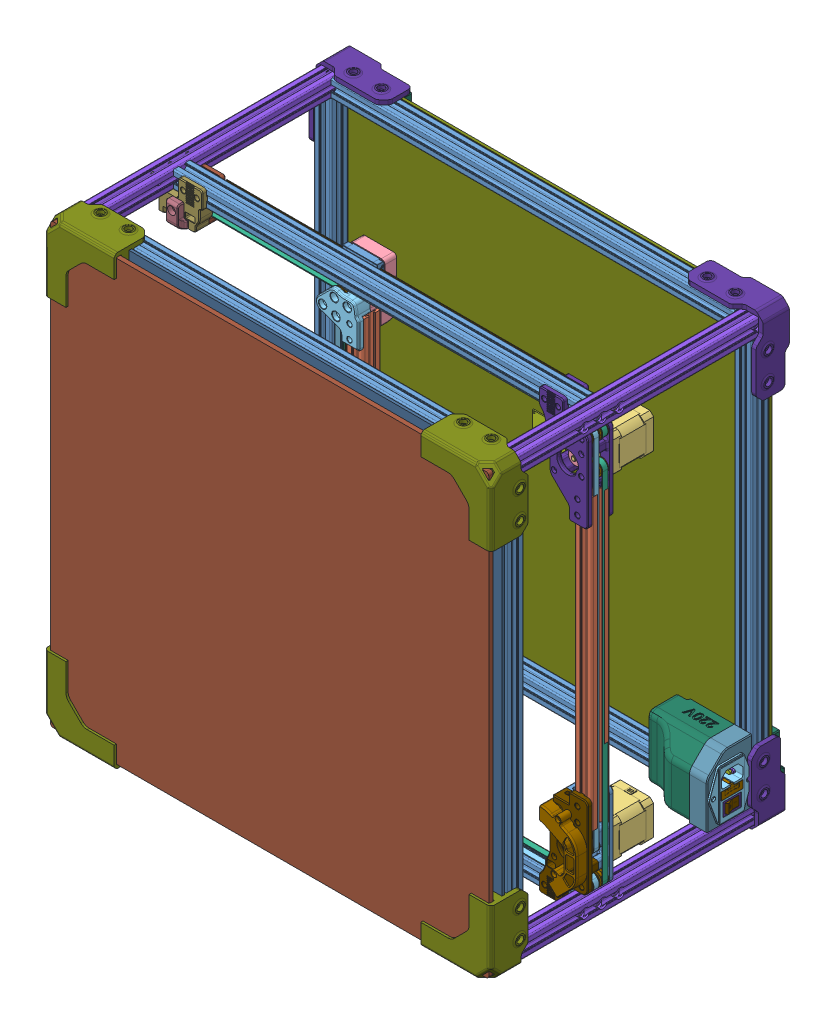
SolidWorks assembly Assem, configuration Default. Lengths in mm. (continued)
Mates (geometry in assembly coordinates): (continued)
- Concentric59: concentric anti-aligned: cylinder of F695 ZZ (1)^Idler Assembly (1)_1_XY Joint - Right_X Axis_Gantry_VORON2 v2.4 Assembly - Final(2)_VORON2 v2.4 Assembly - Final-19 through (240.5064 -184.1733 3) axis (0 0 1) radius 6.5; cylinder of F695 ZZ (1)^Idler Assembly (1)_1_XY Joint - Right_X Axis_Gantry_VORON2 v2.4 Assembly - Final(2)_VORON2 v2.4 Assembly - Final-20 through (240.5064 -184.1733 7) axis (0 0 -1) radius 6.5
- Concentric60: concentric aligned: cylinder of A Drive Frame-23^A Drive Frame_A Drive_Gantry_VORON2 v2.4 Assembly - Final(2)_VORON2 v2.4 Assembly - Final-1 through (240.5064 -184.1733 15) axis (0 0 -1) radius 2.7; cylinder of F695 ZZ (1)^Idler Assembly (1)_1_XY Joint - Right_X Axis_Gantry_VORON2 v2.4 Assembly - Final(2)_VORON2 v2.4 Assembly - Final-20 through (240.5064 -184.1733 7) axis (0 0 -1) radius 6.5
- Coincident93: coincident anti-aligned: plane of A Drive Frame-23^A Drive Frame_A Drive_Gantry_VORON2 v2.4 Assembly - Final(2)_VORON2 v2.4 Assembly - Final-1 through (220.1397 -181.8752 10) normal (0 0 -1); plane of M5 1mm Spacer (1)^Idler Assembly (1)_1_XY Joint - Right_X Axis_Gantry_VORON2 v2.4 Assembly - Final(2)_VORON2 v2.4 Assembly - Final-19 through (240.5064 -184.1733 10) normal (0 0 1)
- Coincident94: coincident anti-aligned: plane of B Drive Frame (1)^B Drive_Gantry_VORON2 v2.4 Assembly - Final(2)_VORON2 v2.4 Assembly - Final-1 through (225.0294 190.9774 -15) normal (0 0 -1); plane of NEMA17 Black^B Drive_Gantry_VORON2 v2.4 Assembly - Final(2)_VORON2 v2.4 Assembly - Final-1 through (204.0284 169.9764 -15) normal (0 0 1)
- Concentric61: concentric anti-aligned: cylinder of B Drive Frame (1)^B Drive_Gantry_VORON2 v2.4 Assembly - Final(2)_VORON2 v2.4 Assembly - Final-1 through (225.0294 190.9774 -16.6) axis (0 0 -1) radius 11.5; cylinder of NEMA17 Black^B Drive_Gantry_VORON2 v2.4 Assembly - Final(2)_VORON2 v2.4 Assembly - Final-1 through (225.0294 190.9774 -15.6) axis (0 0 1) radius 11
- Parallel3: parallel aligned: plane of B Drive Frame (1)^B Drive_Gantry_VORON2 v2.4 Assembly - Final(2)_VORON2 v2.4 Assembly - Final-1 through (248.0294 221.1733 -16.6) normal (1 0 0); plane of NEMA17 Black^B Drive_Gantry_VORON2 v2.4 Assembly - Final(2)_VORON2 v2.4 Assembly - Final-1 through (246.0294 174.1654 -25.161) normal (1 0 0)
- Concentric62: concentric anti-aligned: cylinder of B Drive Frame (1)^B Drive_Gantry_VORON2 v2.4 Assembly - Final(2)_VORON2 v2.4 Assembly - Final-1 through (240.5294 221.1733 15) axis (0 0 1) radius 2.7; cylinder of F695 ZZ (1)^Idler Assembly (1)_1_XY Joint - Right_X Axis_Gantry_VORON2 v2.4 Assembly - Final(2)_VORON2 v2.4 Assembly - Final-16 through (240.5294 221.1733 7) axis (0 0 -1) radius 6.5
- Coincident97: coincident anti-aligned: plane of A Drive Frame-24^A Drive Frame_A Drive_Gantry_VORON2 v2.4 Assembly - Final(2)_VORON2 v2.4 Assembly - Final-1 through (220.0147 -192 -15) normal (0 0 -1); plane of NEMA17 Black^B Drive_Gantry_VORON2 v2.4 Assembly - Final(2)_VORON2 v2.4 Assembly - Final-2 through (246.0304 -169.9764 -15) normal (0 0 1)
- Concentric63: concentric aligned: cylinder of A Drive Frame-24^A Drive Frame_A Drive_Gantry_VORON2 v2.4 Assembly - Final(2)_VORON2 v2.4 Assembly - Final-1 through (225.0294 -190.9774 -16.6) axis (0 0 1) radius 11.5; cylinder of NEMA17 Black^B Drive_Gantry_VORON2 v2.4 Assembly - Final(2)_VORON2 v2.4 Assembly - Final-2 through (225.0294 -190.9774 -15.6) axis (0 0 1) radius 11
- Parallel4: parallel aligned: plane of A Drive Frame-24^A Drive Frame_A Drive_Gantry_VORON2 v2.4 Assembly - Final(2)_VORON2 v2.4 Assembly - Final-1 through (248.0294 -221.1733 -16.6) normal (1 0 0); plane of NEMA17 Black^B Drive_Gantry_VORON2 v2.4 Assembly - Final(2)_VORON2 v2.4 Assembly - Final-2 through (246.0294 -174.1654 -25.161) normal (1 0 0)
- Concentric64: concentric anti-aligned: cylinder of NEMA17 Black^B Drive_Gantry_VORON2 v2.4 Assembly - Final(2)_VORON2 v2.4 Assembly - Final-2 through (225.0294 -190.9774 8.3401) axis (0 0 -1) radius 2.4956; cylinder of GT2 20T 6mm^B Drive_Gantry_VORON2 v2.4 Assembly - Final(2)_VORON2 v2.4 Assembly - Final-1 through (225.0294 -190.9774 -6.35) axis (0 0 1) radius 2.5
- Distance14: distance = 0.5 mm aligned: plane of GT2 20T 6mm^B Drive_Gantry_VORON2 v2.4 Assembly - Final(2)_VORON2 v2.4 Assembly - Final-1 through (225.0294 -190.9774 8.5) normal (0 0 -1); plane of F695 ZZ (1)^Idler Assembly (1)_1_XY Joint - Right_X Axis_Gantry_VORON2 v2.4 Assembly - Final(2)_VORON2 v2.4 Assembly - Final-20 through (240.5064 -184.1733 8) normal (0 0 -1)
- Concentric66: concentric aligned: cylinder of NEMA17 Black^B Drive_Gantry_VORON2 v2.4 Assembly - Final(2)_VORON2 v2.4 Assembly - Final-1 through (225.0294 190.9774 8.3401) axis (0 0 -1) radius 2.4956; cylinder of GT2 20T 6mm^B Drive_Gantry_VORON2 v2.4 Assembly - Final(2)_VORON2 v2.4 Assembly - Final-2 through (225.0294 190.9774 6.35) axis (0 0 -1) radius 2.5
- Distance15: distance = 0.5 mm aligned: plane of GT2 20T 6mm^B Drive_Gantry_VORON2 v2.4 Assembly - Final(2)_VORON2 v2.4 Assembly - Final-2 through (225.0294 190.9774 -1.5) normal (0 0 -1); plane of F695 ZZ (1)^Idler Assembly (1)_1_XY Joint - Right_X Axis_Gantry_VORON2 v2.4 Assembly - Final(2)_VORON2 v2.4 Assembly - Final-17 through (240.5064 184.1733 -2) normal (0 0 -1)
- Coincident102: coincident anti-aligned: plane of Front Idler B Bottom^Front Idler B_Gantry_VORON2 v2.4 Assembly - Final(2)_VORON2 v2.4 Assembly - Final-1 through (-220 227.6989 -10) normal (0 0 1); plane of M5 1mm Spacer (1)^Idler Assembly (1)_1_XY Joint - Right_X Axis_Gantry_VORON2 v2.4 Assembly - Final(2)_VORON2 v2.4 Assembly - Final-5 through (-219.5002 221.0003 -10) normal (0 0 -1)
- BeltMate1: belt = 13 : 12.22 mm: cylinder of GT2 20T 6mm^B Drive_Gantry_VORON2 v2.4 Assembly - Final(2)_VORON2 v2.4 Assembly - Final-2 through (225.0294 190.9774 6.35) axis (0 0 1) radius 6.11; cylinder of F695 ZZ (1)^Idler Assembly (1)_1_XY Joint - Right_X Axis_Gantry_VORON2 v2.4 Assembly - Final(2)_VORON2 v2.4 Assembly - Final-18 through (240.5064 184.1733 -7) axis (0 0 1) radius 6.5
- BeltMate2: belt = 13 : 13 mm: cylinder of F695 ZZ (1)^Idler Assembly (1)_1_XY Joint - Right_X Axis_Gantry_VORON2 v2.4 Assembly - Final(2)_VORON2 v2.4 Assembly - Final-18 through (240.5064 184.1733 -7) axis (0 0 1) radius 6.5; cylinder of F695 ZZ (1)^Idler Assembly (1)_1_XY Joint - Right_X Axis_Gantry_VORON2 v2.4 Assembly - Final(2)_VORON2 v2.4 Assembly - Final-12 through (240.5294 -221.1733 -3) axis (0 0 -1) radius 6.5
- BeltMate3: belt = 13 : 13 mm: cylinder of F695 ZZ (1)^Idler Assembly (1)_1_XY Joint - Right_X Axis_Gantry_VORON2 v2.4 Assembly - Final(2)_VORON2 v2.4 Assembly - Final-12 through (240.5294 -221.1733 -3) axis (0 0 -1) radius 6.5; cylinder of F695 ZZ (1)^Idler Assembly (1)_1_XY Joint - Right_X Axis_Gantry_VORON2 v2.4 Assembly - Final(2)_VORON2 v2.4 Assembly - Final-2 through (-40.7546 -221.05 -3.3) axis (0 0 -1) radius 6.5
- BeltMate4: belt = 12.22 : 13 mm: cylinder of F695 ZZ (1)^Idler Assembly (1)_1_XY Joint - Right_X Axis_Gantry_VORON2 v2.4 Assembly - Final(2)_VORON2 v2.4 Assembly - Final-2 through (-40.7546 -221.05 -3.3) axis (0 0 -1) radius 6.5; cylinder of GT2 20T Idler Gates v2^XY Joint - Right_X Axis_Gantry_VORON2 v2.4 Assembly - Final(2)_VORON2 v2.4 Assembly - Final-2 through (-53.9146 207.89 -17) axis (0 0 -1) radius 6.11
- BeltMate5: belt = 13 : 12.22 mm: cylinder of GT2 20T Idler Gates v2^XY Joint - Right_X Axis_Gantry_VORON2 v2.4 Assembly - Final(2)_VORON2 v2.4 Assembly - Final-2 through (-53.9146 207.89 -17) axis (0 0 -1) radius 6.11; cylinder of F695 ZZ (1)^Idler Assembly (1)_1_XY Joint - Right_X Axis_Gantry_VORON2 v2.4 Assembly - Final(2)_VORON2 v2.4 Assembly - Final-6 through (-219.5002 221.0003 -7) axis (0 0 1) radius 6.5
- BeltMate6: belt = 13 : 13 mm: cylinder of F695 ZZ (1)^Idler Assembly (1)_1_XY Joint - Right_X Axis_Gantry_VORON2 v2.4 Assembly - Final(2)_VORON2 v2.4 Assembly - Final-6 through (-219.5002 221.0003 -7) axis (0 0 1) radius 6.5; cylinder of F695 ZZ (1)^Idler Assembly (1)_1_XY Joint - Right_X Axis_Gantry_VORON2 v2.4 Assembly - Final(2)_VORON2 v2.4 Assembly - Final-13 through (240.5294 221.1733 -3) axis (0 0 -1) radius 6.5
- BeltMate7: belt = 13 : 12.22 mm: cylinder of GT2 20T 6mm^B Drive_Gantry_VORON2 v2.4 Assembly - Final(2)_VORON2 v2.4 Assembly - Final-1 through (225.0294 -190.9774 -6.35) axis (0 0 -1) radius 6.11; cylinder of F695 ZZ (1)^Idler Assembly (1)_1_XY Joint - Right_X Axis_Gantry_VORON2 v2.4 Assembly - Final(2)_VORON2 v2.4 Assembly - Final-19 through (240.5064 -184.1733 3) axis (0 0 1) radius 6.5
- BeltMate8: belt = 13 : 13 mm: cylinder of F695 ZZ (1)^Idler Assembly (1)_1_XY Joint - Right_X Axis_Gantry_VORON2 v2.4 Assembly - Final(2)_VORON2 v2.4 Assembly - Final-19 through (240.5064 -184.1733 3) axis (0 0 1) radius 6.5; cylinder of F695 ZZ (1)^Idler Assembly (1)_1_XY Joint - Right_X Axis_Gantry_VORON2 v2.4 Assembly - Final(2)_VORON2 v2.4 Assembly - Final-15 through (240.5294 221.1733 3) axis (0 0 1) radius 6.5
- BeltMate9: belt = 13 : 13 mm: cylinder of F695 ZZ (1)^Idler Assembly (1)_1_XY Joint - Right_X Axis_Gantry_VORON2 v2.4 Assembly - Final(2)_VORON2 v2.4 Assembly - Final-15 through (240.5294 221.1733 3) axis (0 0 1) radius 6.5; cylinder of F695 ZZ (1)^Idler Assembly (1)_1_XY Joint - Right_X Axis_Gantry_VORON2 v2.4 Assembly - Final(2)_VORON2 v2.4 Assembly - Final-3 through (-40.7546 221.05 6.7) axis (0 0 -1) radius 6.5
- BeltMate10: belt = 12.22 : 13 mm: cylinder of F695 ZZ (1)^Idler Assembly (1)_1_XY Joint - Right_X Axis_Gantry_VORON2 v2.4 Assembly - Final(2)_VORON2 v2.4 Assembly - Final-3 through (-40.7546 221.05 6.7) axis (0 0 -1) radius 6.5; cylinder of GT2 20T Idler Gates v2^XY Joint - Right_X Axis_Gantry_VORON2 v2.4 Assembly - Final(2)_VORON2 v2.4 Assembly - Final-1 through (-53.9146 -207.89 -7) axis (0 0 -1) radius 6.11
- BeltMate11: belt = 13 : 12.22 mm: cylinder of GT2 20T Idler Gates v2^XY Joint - Right_X Axis_Gantry_VORON2 v2.4 Assembly - Final(2)_VORON2 v2.4 Assembly - Final-1 through (-53.9146 -207.89 -7) axis (0 0 -1) radius 6.11; cylinder of F695 ZZ (1)^Idler Assembly (1)_1_XY Joint - Right_X Axis_Gantry_VORON2 v2.4 Assembly - Final(2)_VORON2 v2.4 Assembly - Final-8 through (-219.5002 -221.0003 7) axis (0 0 -1) radius 6.5
- BeltMate12: belt = 13 : 13 mm: cylinder of F695 ZZ (1)^Idler Assembly (1)_1_XY Joint - Right_X Axis_Gantry_VORON2 v2.4 Assembly - Final(2)_VORON2 v2.4 Assembly - Final-8 through (-219.5002 -221.0003 7) axis (0 0 -1) radius 6.5; cylinder of F695 ZZ (1)^Idler Assembly (1)_1_XY Joint - Right_X Axis_Gantry_VORON2 v2.4 Assembly - Final(2)_VORON2 v2.4 Assembly - Final-10 through (240.5294 -221.1733 3) axis (0 0 1) radius 6.5
- LockToSketchMate2: unknown: line of Belt1-5-1 through (220.0294 190.9774 -5) axis (1 0 0); line of Belt1-5-1 through (220.0294 190.9774 -5) axis (0 1 0)
- Coincident103: coincident anti-aligned: plane of ALP2020_460-4 through (-230 -230 108.5) normal (1 0 0); plane of ALP2020_460-6 through (-230 -234.1 97.9891) normal (-1 0 0)
- Coincident104: coincident aligned: plane of ALP2020_460-4 through (-236.1 -230 110) normal (0 0 1); plane of ALP2020_460-6 through (230 -236.1 110) normal (0 0 1)
- Coincident105: coincident aligned: plane of ALP2020_460-5 through (243.9 -230 110) normal (0 0 1); plane of ALP2020_460-6 through (230 -236.1 110) normal (0 0 1)
- Coincident106: coincident anti-aligned: plane of ALP2020_460-5 through (245.9 -230 97.9891) normal (0 -1 0); plane of ALP2020_460-6 through (230 -230 108.5) normal (0 1 0)
- Coincident107: coincident aligned: plane of ALP2020_460-3 through (230 231.5 110) normal (0 0 1); plane of ALP2020_460-5 through (231.5 -230 110) normal (0 0 1)
- Coincident108: coincident anti-aligned: plane of ALP2020_460-3 through (230 245.9 97.9891) normal (1 0 0); plane of ALP2020_460-5 through (230 -230 103.9) normal (-1 0 0)
- Coincident109: coincident anti-aligned: plane of ALP2020_460-3 through (230 230 103.9) normal (0 -1 0); plane of ALP2020_460-5 through (245.9 230 97.9891) normal (0 1 0)
- Coincident110: coincident anti-aligned: plane of ALP2020_460-3 through (230 230 103.9) normal (0 -1 0); plane of ALP2020_460-4 through (-234.1 230 97.9891) normal (0 1 0)
- Coincident113: coincident anti-aligned: plane of ALP2020_460-5 through (230 -230 103.9) normal (-1 0 0); plane of ALP2020_460-6 through (230 -234.1 97.9891) normal (1 0 0)
- Coincident114: coincident aligned: plane of ALP2020_460-1 through (230 250 8.5) normal (0 1 0); plane of ALP2020_460-3 through (230 250 108.5) normal (0 1 0)
- Coincident115: coincident aligned: plane of ALP2020_460-1 through (230 245.9 -2.0109) normal (1 0 0); plane of ALP2020_460-3 through (230 245.9 97.9891) normal (1 0 0)
- Coincident116: coincident anti-aligned: plane of ALP2020_460-7 through (-230 -230 -171.5) normal (1 0 0); plane of ALP2020_460-8 through (-230 -234.1 -182.0109) normal (-1 0 0)
- Coincident117: coincident aligned: plane of ALP2020_460-7 through (-236.1 -230 -170) normal (0 0 1); plane of ALP2020_460-8 through (230 -236.1 -170) normal (0 0 1)
- Coincident118: coincident anti-aligned: plane of ALP2020_460-9 through (230 -230 -176.1) normal (-1 0 0); plane of ALP2020_460-10 through (230 245.9 -182.0109) normal (1 0 0)
- Coincident119: coincident aligned: plane of ALP2020_460-8 through (230 -236.1 -170) normal (0 0 1); plane of ALP2020_460-9 through (243.9 -230 -170) normal (0 0 1)
- Coincident120: coincident anti-aligned: plane of ALP2020_460-7 through (-234.1 230 -182.0109) normal (0 1 0); plane of ALP2020_460-10 through (230 230 -176.1) normal (0 -1 0)
- Coincident121: coincident anti-aligned: plane of ALP2020_460-9 through (245.9 230 -182.0109) normal (0 1 0); plane of ALP2020_460-10 through (230 230 -176.1) normal (0 -1 0)
- Coincident122: coincident aligned: plane of ALP2020_460-9 through (231.5 -230 -170) normal (0 0 1); plane of ALP2020_460-10 through (230 231.5 -170) normal (0 0 1)
- Coincident123: coincident anti-aligned: plane of ALP2020_460-8 through (230 -230 -171.5) normal (0 1 0); plane of ALP2020_460-9 through (245.9 -230 -182.0109) normal (0 -1 0)
- Coincident124: coincident anti-aligned: plane of ALP2020_460-8 through (230 -234.1 -182.0109) normal (1 0 0); plane of ALP2020_460-9 through (230 -230 -176.1) normal (-1 0 0)
- Coincident125: coincident aligned: plane of ALP2020_460-1 through (230 250 8.5) normal (0 1 0); plane of ALP2020_460-10 through (230 250 -171.5) normal (0 1 0)
- Coincident126: coincident aligned: plane of ALP2020_460-1 through (230 245.9 -2.0109) normal (1 0 0); plane of ALP2020_460-10 through (230 245.9 -182.0109) normal (1 0 0)
- Distance16: distance = 80 mm anti-aligned: plane of ALP2020_460-6 through (230 -243.9 90) normal (0 0 -1); plane of ALP2020_460-2 through (230 -248.5 10) normal (0 0 1)
- Coincident127: coincident aligned: plane of ALP2020_460-8 through (230 -231.5 -190) normal (0 0 -1); plane of camera-1 through (-5.0058 -4.6135 -190) normal (0 0 -1)
- Coincident128: coincident: line of camera-1 through (0 0 -171.4) axis (0 0 -1)
- Parallel5: parallel aligned: plane of ALP2020_460-7 through (-250 -230 -176.1) normal (-1 0 0); plane of camera-1 through (-6.5 -6.5 -180) normal (-1 0 0)
- Distance17: distance = 300 mm anti-aligned: plane of ALP2020_460-3 through (230 243.9 110) normal (0 0 1); plane of ALP2020_460-10 through (230 248.5 -190) normal (0 0 -1)
- Coincident130: coincident aligned: plane of ALP2020_300-5 through (242.0109 234.1 110) normal (0 0 1); plane of ALP2020_300-4 through (242.0109 -245.9 110) normal (0 0 1)
- Coincident131: coincident aligned: plane of ALP2020_300-5 through (242.0109 234.1 110) normal (0 0 1); plane of ALP2020_300-2 through (-242.0109 245.9 110) normal (0 0 1)
- Coincident132: coincident aligned: plane of ALP2020_300-5 through (242.0109 234.1 110) normal (0 0 1); plane of ALP2020_300-1 through (-242.0109 -234.1 110) normal (0 0 1)
- Coincident133: coincident aligned: plane of ALP2020_300-5 through (242.0109 234.1 110) normal (0 0 1); plane of ALP2020_460-3 through (230 231.5 110) normal (0 0 1)
- Coincident134: coincident aligned: plane of ALP2020_460-3 through (230 250 108.5) normal (0 1 0); plane of ALP2020_300-2 through (-243.9 250 -190) normal (0 1 0)
- Coincident135: coincident aligned: plane of ALP2020_460-4 through (-250 -230 103.9) normal (-1 0 0); plane of ALP2020_300-2 through (-250 248.5 -190) normal (-1 0 0)
- Coincident140: coincident aligned: plane of ALP2020_460-6 through (230 -250 91.5) normal (0 -1 0); plane of ALP2020_300-1 through (-236.1 -250 -190) normal (0 -1 0)
- Coincident141: coincident aligned: plane of ALP2020_460-4 through (-250 -230 91.5) normal (-1 0 0); plane of ALP2020_300-1 through (-250 -243.9 -190) normal (-1 0 0)
- Coincident142: coincident anti-aligned: plane of A Drive Frame-23^A Drive Frame_A Drive_Gantry_VORON2 v2.4 Assembly - Final(2)_VORON2 v2.4 Assembly - Final-1 through (220.0147 -192 15) normal (0 0 1); plane of cable cover^A Drive_Gantry_VORON2 v2.4 Assembly - Final(2)_VORON2 v2.4 Assembly - Final-1 through (223.0748 -195.8252 15) normal (0 0 -1)
- Concentric67: concentric anti-aligned: cylinder of A Drive Frame-23^A Drive Frame_A Drive_Gantry_VORON2 v2.4 Assembly - Final(2)_VORON2 v2.4 Assembly - Final-1 through (221.5428 -212.1725 15) axis (0 0 -1) radius 2.35; cylinder of cable cover^A Drive_Gantry_VORON2 v2.4 Assembly - Final(2)_VORON2 v2.4 Assembly - Final-1 through (221.5428 -212.1725 21) axis (0 0 1) radius 1.7
- Concentric68: concentric aligned: cylinder of A Drive Frame-23^A Drive Frame_A Drive_Gantry_VORON2 v2.4 Assembly - Final(2)_VORON2 v2.4 Assembly - Final-1 through (225.7197 -156.0933 15) axis (0 0 -1) radius 2.35; cylinder of cable cover^A Drive_Gantry_VORON2 v2.4 Assembly - Final(2)_VORON2 v2.4 Assembly - Final-1 through (225.7197 -156.0933 27) axis (0 0 -1) radius 3
- Coincident143: coincident aligned: plane of ALP2020_460-5 through (250 -230 108.5) normal (1 0 0); plane of ALP2020_300-4 through (250 -236.1 -190) normal (1 0 0)
- Coincident144: coincident aligned: plane of ALP2020_460-6 through (230 -250 103.9) normal (0 -1 0); plane of ALP2020_300-4 through (243.9 -250 -190) normal (0 -1 0)
- Coincident145: coincident aligned: plane of ALP2020_460-5 through (250 -230 108.5) normal (1 0 0); plane of ALP2020_300-5 through (250 231.5 -190) normal (1 0 0)
- Coincident146: coincident aligned: plane of ALP2020_460-3 through (230 250 96.1) normal (0 1 0); plane of ALP2020_300-5 through (236.1 250 -190) normal (0 1 0)
- Distance18: distance = 2 mm anti-aligned: plane of GlassSheet3mm-1 through (0 0 112) normal (0 0 -1); plane of ALP2020_460-3 through (230 231.5 110) normal (0 0 1)
- Coincident185: coincident aligned: plane of ALP2020_460-3 through (230 250 108.5) normal (0 1 0); plane of GlassSheet3mm-1 through (-250 250 112) normal (0 1 0)
- Coincident186: coincident aligned: plane of ALP2020_460-5 through (250 -230 108.5) normal (1 0 0); plane of GlassSheet3mm-1 through (250 -250 112) normal (1 0 0)
- Distance21: distance = 10 mm anti-aligned: plane of GlassSheet5mm-1 through (0 0 125) normal (0 0 -1); plane of GlassSheet3mm-1 through (0 0 115) normal (0 0 1)
- Coincident151: coincident aligned: plane of GlassSheet3mm-1 through (-250 250 112) normal (0 1 0); plane of GlassSheet5mm-1 through (-250 250 125) normal (0 1 0)
- Coincident152: coincident aligned: plane of GlassSheet3mm-1 through (250 -250 112) normal (1 0 0); plane of GlassSheet5mm-1 through (250 -250 125) normal (1 0 0)
- Coincident168: coincident aligned: plane of ALP2020_460-10 through (230 250 -183.9) normal (0 1 0); plane of FootCorner-1 through (-250 250 -203) normal (0 1 0)
- Distance22: distance = 3 mm anti-aligned: plane of FootCorner-1 through (-230 230 -193) normal (0 0 1); plane of ALP2020_460-7 through (-243.9 -230 -190) normal (0 0 -1)
- Coincident170: coincident aligned: plane of ALP2020_460-7 through (-250 -230 -188.5) normal (-1 0 0); plane of FootCorner-1 through (-250 170 -203) normal (-1 0 0)
- Coincident171: coincident aligned: plane of ALP2020_460-9 through (250 -230 -183.9) normal (1 0 0); plane of FootCorner-2 through (250 250 -203) normal (1 0 0)
- Coincident172: coincident aligned: plane of ALP2020_460-10 through (230 250 -183.9) normal (0 1 0); plane of FootCorner-2 through (170 250 -203) normal (0 1 0)
- Coincident173: coincident aligned: plane of FootCorner-1 through (-230 230 -193) normal (0 0 1); plane of FootCorner-2 through (230 230 -193) normal (0 0 1)
- Coincident174: coincident aligned: plane of FootCorner-2 through (230 230 -193) normal (0 0 1); plane of FootCorner-4 through (230 -230 -193) normal (0 0 1)
- Coincident175: coincident aligned: plane of ALP2020_460-9 through (250 -230 -183.9) normal (1 0 0); plane of FootCorner-4 through (250 -170 -203) normal (1 0 0)
- Coincident176: coincident aligned: plane of ALP2020_460-8 through (230 -250 -188.5) normal (0 -1 0); plane of FootCorner-4 through (250 -250 -203) normal (0 -1 0)
- Coincident177: coincident aligned: plane of FootCorner-1 through (-230 230 -193) normal (0 0 1); plane of FootCorner-3 through (-230 -230 -193) normal (0 0 1)
- Coincident178: coincident aligned: plane of ALP2020_460-7 through (-250 -230 -188.5) normal (-1 0 0); plane of FootCorner-3 through (-250 -250 -203) normal (-1 0 0)
- Coincident179: coincident aligned: plane of ALP2020_460-8 through (230 -250 -188.5) normal (0 -1 0); plane of FootCorner-3 through (-170 -250 -203) normal (0 -1 0)
- InPlace1: in place: plane of ALP2020_460-10 through (230 248.5 -190) normal (0 0 -1); plane of ? through (0 0 -190) normal (0 0 -1); moOrthogonalPlaneRef_w of ALP2020_460-10 through (230 248.5 -190) normal (0 0 -1); plane of ? through (0 0 -190) normal (0 1 0); plane of ALP2020_460-10 through (230 248.5 -190) normal (0 0 -1); plane of ? through (0 0 -190) normal (-1 0 0); plane of ALP2020_460-10 through (230 248.5 -190) normal (0 0 -1); unknown of BottomAcrylicPanel-1
- Coincident180: coincident aligned: plane of ALP2020_460-10; plane of BottomAcrylicPanel-1
- Coincident181: coincident aligned: plane of ALP2020_460-10 through (0 240 -190) normal (0 1 0); plane of Part1^Assem-1 through (0 240 -190) normal (0 1 0)
- Coincident182: coincident anti-aligned: plane of ALP2020_460-10 through (0 240 -190) normal (1 0 0); plane of Part1^Assem-1 through (0 240 -190) normal (-1 0 0)
- Coincident180: coincident anti-aligned: plane of ALP2020_300-4 through (250 -236.1 -190) normal (1 0 0); plane of IEC320-C14-1/IEC320-C14.STEP-1/ilpm_case.STEP-1 through (250 -198.55 -165.2433) normal (-1 0 0)
- Distance23: distance = 12 mm anti-aligned: plane of IEC320-C14-1/IEC320-C14.STEP-1/ilpm_case.STEP-1 through (232.5 -181.1 -158) normal (0 0 -1); plane of ALP2020_460-9 through (243.9 -230 -170) normal (0 0 1)
- Distance24: distance = 8 mm anti-aligned: plane of IEC320-C14-1/IEC320-C14.STEP-1/ilpm_case.STEP-1 through (232.5 -222 -156) normal (0 -1 0); plane of ALP2020_300-4 through (248.5 -230 -190) normal (0 1 0)
- InPlace3: in place: plane of ? through (250 -198.55 -165.2433) normal (-1 0 0); plane of ? through (250 0 0) normal (-1 0 0); plane of ? through (250 -198.55 -165.2433) normal (-1 0 0); plane of ? through (250 0 0) normal (0 1 0); plane of ? through (250 -198.55 -165.2433) normal (-1 0 0); plane of ? through (250 0 0) normal (0 0 1); plane of ? through (250 -198.55 -165.2433) normal (-1 0 0); unknown of ?
- Coincident186: coincident aligned: plane of ?; plane of PowerSwitchMount-1
- Coincident187: coincident aligned: plane of IEC320-C14-1/IEC320-C14.STEP-1/ilpm_case.STEP-1 through (250 -198.55 -144.5) normal (0 1 0); plane of Part2^Assem-1 through (250 -198.55 -144.5) normal (0 1 0)
- Coincident188: coincident anti-aligned: plane of IEC320-C14-1/IEC320-C14.STEP-1/ilpm_case.STEP-1 through (250 -198.55 -144.5) normal (0 0 -1); plane of Part2^Assem-1 through (250 -198.55 -144.5) normal (0 0 1)
- InPlace4: in place: plane of ? through (230 -198.55 -144.5) normal (-1 0 0); plane of ? through (230 0 0) normal (-1 0 0); plane of ? through (230 -198.55 -144.5) normal (-1 0 0); plane of ? through (230 0 0) normal (0 1 0); plane of ? through (230 -198.55 -144.5) normal (-1 0 0); plane of ? through (230 0 0) normal (0 0 1); plane of ? through (230 -198.55 -144.5) normal (-1 0 0); unknown of PowerCover-1
- Coincident189: coincident aligned: plane of PowerSwitchMount-1; plane of PowerCover-1
- Coincident190: coincident aligned: plane of PowerSwitchMount-1 through (230 -198.55 -144.5) normal (0 1 0); plane of PowerCover-1 through (230 -198.55 -144.5) normal (0 1 0)
- Coincident191: coincident anti-aligned: plane of PowerSwitchMount-1 through (230 -198.55 -144.5) normal (0 0 -1); plane of PowerCover-1 through (230 -198.55 -144.5) normal (0 0 1)
- Coincident181: coincident anti-aligned: plane of X Carriage Frame-36^X Carriage Frame_X Carriage_X Axis_Gantry_VORON2 v2.4 Assembly - Final(2)_VORON2 v2.4 Assembly - Final-1 through (-48.3904 -39.2904 14.5771) normal (0 1 0); plane of X Carriage Frame-35^X Carriage Frame_X Carriage_X Axis_Gantry_VORON2 v2.4 Assembly - Final(2)_VORON2 v2.4 Assembly - Final-1 through (-48.3904 -39.2904 14.5771) normal (0 -1 0)
- Coincident182: coincident aligned: plane of X Carriage Frame-36^X Carriage Frame_X Carriage_X Axis_Gantry_VORON2 v2.4 Assembly - Final(2)_VORON2 v2.4 Assembly - Final-1 through (-38.0904 -34.1654 -16.5925) normal (1 0 0); plane of X Carriage Frame-35^X Carriage Frame_X Carriage_X Axis_Gantry_VORON2 v2.4 Assembly - Final(2)_VORON2 v2.4 Assembly - Final-1 through (-38.0904 -34.1654 -16.5925) normal (1 0 0)
- Coincident183: coincident aligned: plane of X Carriage Frame-35^X Carriage Frame_X Carriage_X Axis_Gantry_VORON2 v2.4 Assembly - Final(2)_VORON2 v2.4 Assembly - Final-1 through (-58.6904 -28.0904 -38.899) normal (0 0 -1); plane of X Carriage Frame-36^X Carriage Frame_X Carriage_X Axis_Gantry_VORON2 v2.4 Assembly - Final(2)_VORON2 v2.4 Assembly - Final-1 through (-106.1195 89.2516 -38.899) normal (0 0 -1)
- Coincident184: coincident anti-aligned: plane of X Carriage Frame-36^X Carriage Frame_X Carriage_X Axis_Gantry_VORON2 v2.4 Assembly - Final(2)_VORON2 v2.4 Assembly - Final-1 through (-60.6904 -52.7904 -1.1995) normal (0 1 0); plane of Belt Clamp_1-34^Belt Clamp_1_X Carriage Frame_X Carriage_X Axis_Gantry_VORON2 v2.4 Assembly - Final(2)_VORON2 v2.4 Assembly - Final-1 through (-50.0904 -52.7904 -9.3995) normal (0 -1 0)
- Concentric69: concentric aligned: cylinder of X Carriage Frame-36^X Carriage Frame_X Carriage_X Axis_Gantry_VORON2 v2.4 Assembly - Final(2)_VORON2 v2.4 Assembly - Final-1 through (-55.2904 -19.2904 -0.3) axis (0 -1 0) radius 1.7; cylinder of Belt Clamp_1-34^Belt Clamp_1_X Carriage Frame_X Carriage_X Axis_Gantry_VORON2 v2.4 Assembly - Final(2)_VORON2 v2.4 Assembly - Final-1 through (-55.2904 -46.6904 -0.3) axis (0 -1 0) radius 2.5
- Parallel6: parallel aligned: plane of X Carriage Frame-36^X Carriage Frame_X Carriage_X Axis_Gantry_VORON2 v2.4 Assembly - Final(2)_VORON2 v2.4 Assembly - Final-1 through (-60.6904 -24.9904 -5.8995) normal (-1 0 0); plane of Belt Clamp_1-34^Belt Clamp_1_X Carriage Frame_X Carriage_X Axis_Gantry_VORON2 v2.4 Assembly - Final(2)_VORON2 v2.4 Assembly - Final-1 through (-59.6904 -51.7404 -10.4237) normal (-1 0 0)
- Coincident187: coincident anti-aligned: plane of ALP2020_460-6 through (230 -250 103.9) normal (0 -1 0); plane of GlassSheetHolderCorner2-1 through (-175 -250 90) normal (0 1 0)
- Coincident188: coincident anti-aligned: plane of ALP2020_460-4 through (-250 -230 103.9) normal (-1 0 0); plane of GlassSheetHolderCorner2-1 through (-250 -250 90) normal (1 0 0)
- Coincident189: coincident anti-aligned: plane of ALP2020_460-4 through (-248.5 -230 110) normal (0 0 1); plane of GlassSheetHolderCorner2-1 through (-230 -230 110) normal (0 0 -1)
- InPlace5: in place: plane of ALP2020_460-7 through (-250 -230 -188.5) normal (-1 0 0); plane of ? through (-250 0 0) normal (-1 0 0); plane of ALP2020_460-7 through (-250 -230 -188.5) normal (-1 0 0); plane of ? through (-250 0 0) normal (0 1 0); plane of ALP2020_460-7 through (-250 -230 -188.5) normal (-1 0 0); plane of ? through (-250 0 0) normal (0 0 1); plane of ALP2020_460-7 through (-250 -230 -188.5) normal (-1 0 0); unknown of BottomCorner-1
- Coincident190: coincident aligned: plane of assembly through (-250 0 -180) normal (-1 0 0)
- Coincident191: coincident aligned: plane of ALP2020_460-7 through (-250 0 -180) normal (0 0 -1); plane of BottomCorner-1 through (-250 0 -180) normal (0 0 -1)
- Coincident192: coincident anti-aligned: plane of ALP2020_460-7 through (-250 0 -180) normal (0 -1 0); plane of BottomCorner-1 through (-250 0 -180) normal (0 1 0)
- Coincident193: coincident anti-aligned: plane of ALP2020_460-7 through (-250 -230 -188.5) normal (-1 0 0); plane of BottomCorner-4 through (-250 0 -180) normal (1 0 0)
- Coincident194: coincident anti-aligned: plane of ALP2020_460-10 through (230 250 -171.5) normal (0 1 0); plane of BottomCorner-4 through (0 250 -180) normal (0 -1 0)
- Coincident195: coincident aligned: plane of FootCorner-1 through (-230 230 -208) normal (0 0 -1); plane of BottomCorner-4 through (-210 255 -208) normal (0 0 -1)
- Coincident196: coincident anti-aligned: plane of ALP2020_460-10 through (230 250 -171.5) normal (0 1 0); plane of BottomCorner-3 through (0 250 -180) normal (0 -1 0)
- Coincident197: coincident anti-aligned: plane of ALP2020_460-9 through (250 -230 -183.9) normal (1 0 0); plane of BottomCorner-3 through (250 0 -180) normal (-1 0 0)
- Coincident198: coincident aligned: plane of FootCorner-2 through (230 230 -208) normal (0 0 -1); plane of BottomCorner-3 through (255 210 -208) normal (0 0 -1)
- Coincident199: coincident anti-aligned: plane of ALP2020_460-8 through (230 -250 -188.5) normal (0 -1 0); plane of BottomCorner-2 through (0 -250 -175) normal (0 1 0)
- Coincident200: coincident anti-aligned: plane of ALP2020_460-9 through (250 -230 -183.9) normal (1 0 0); plane of BottomCorner-2 through (250 0 -175) normal (-1 0 0)
- Coincident201: coincident aligned: plane of FootCorner-4 through (230 -230 -203) normal (0 0 -1); plane of BottomCorner-2 through (210 -255 -203) normal (0 0 -1)
- Coincident202: coincident anti-aligned: plane of ALP2020_460-6 through (230 -250 103.9) normal (0 -1 0); plane of GlassSheetHolderCorner2-2 through (250 -250 90) normal (0 1 0)
- Coincident203: coincident anti-aligned: plane of ALP2020_460-5 through (250 -230 96.1) normal (1 0 0); plane of GlassSheetHolderCorner2-2 through (250 -175 90) normal (-1 0 0)
- Coincident204: coincident anti-aligned: plane of ALP2020_460-6 through (230 -248.5 110) normal (0 0 1); plane of GlassSheetHolderCorner2-2 through (230 -230 110) normal (0 0 -1)
- Coincident205: coincident anti-aligned: plane of ALP2020_460-4 through (-250 -230 91.5) normal (-1 0 0); plane of GlassSheetHolderCorner2-3 through (-250 175 90) normal (1 0 0)
- Coincident206: coincident anti-aligned: plane of ALP2020_460-3 through (230 250 96.1) normal (0 1 0); plane of GlassSheetHolderCorner2-3 through (-250 250 90) normal (0 -1 0)
- Coincident207: coincident anti-aligned: plane of ALP2020_460-3 through (230 243.9 110) normal (0 0 1); plane of GlassSheetHolderCorner2-3 through (-230 230 110) normal (0 0 -1)
- Coincident208: coincident anti-aligned: plane of ALP2020_460-5 through (250 -230 96.1) normal (1 0 0); plane of GlassSheetHolderCorner2-4 through (250 250 90) normal (-1 0 0)
- Coincident209: coincident anti-aligned: plane of ALP2020_460-3 through (230 250 96.1) normal (0 1 0); plane of GlassSheetHolderCorner2-4 through (175 250 90) normal (0 -1 0)
- Coincident210: coincident anti-aligned: plane of ALP2020_460-3 through (230 243.9 110) normal (0 0 1); plane of GlassSheetHolderCorner2-4 through (230 230 110) normal (0 0 -1)
- Coincident212: coincident anti-aligned: plane of ALP2020_460-1 through (230 248.5 -10) normal (0 0 -1); plane of MGN9-250-1/MGN9-1 through (195 244.3 -10) normal (0 0 1)
- Distance25: distance = 5.5 mm aligned: plane of MGN9-250-1/MGN9-1 through (195 244.5 -10.2) normal (0 1 0); plane of ALP2020_460-1 through (230 250 -3.9) normal (0 1 0)
- Coincident215: coincident anti-aligned: plane of B Drive Frame (1)^B Drive_Gantry_VORON2 v2.4 Assembly - Final(2)_VORON2 v2.4 Assembly - Final-1 through (195 242.245 -10) normal (-1 0 0); plane of MGN9-250-1/MGN9-1 through (195 244.6 -14.7) normal (1 0 0)
- Coincident216: coincident aligned: plane of XY Joint - Left-56^XY Joint - Left_X Axis_Gantry_VORON2 v2.4 Assembly - Final(2)_VORON2 v2.4 Assembly - Final-1 through (-19.2404 250 -34.3) normal (1 0 0); plane of MGN9-250-1/MGN9-H-1 through (-19.2404 240 -16) normal (1 0 0)
- Coincident217: coincident anti-aligned: plane of ALP2020_460-2 through (230 -243.9 -10) normal (0 0 -1); plane of MGN9-390-2/MGN9-1 through (195 -235.7 -10) normal (0 0 1)
- Distance26: distance = 5.5 mm aligned: plane of MGN9-390-2/MGN9-1 through (195 -244.5 -10.2) normal (0 -1 0); plane of ALP2020_460-2 through (230 -250 3.9) normal (0 -1 0)
- Coincident219: coincident anti-aligned: plane of A Drive Frame-24^A Drive Frame_A Drive_Gantry_VORON2 v2.4 Assembly - Final(2)_VORON2 v2.4 Assembly - Final-1 through (195 -242.245 -10) normal (-1 0 0); plane of MGN9-390-2/MGN9-1 through (195 -235.4 -14.7) normal (1 0 0)
- Coincident220: coincident anti-aligned: plane of ALP2020_420-1 through (-33.2904 210 8.2) normal (-1 0 0); plane of MGN9-390-3/MGN9-1 through (-33.2904 194.9 4) normal (1 0 0)
- Distance27: distance = 5.5 mm aligned: plane of MGN9-390-3/MGN9-1 through (-33.4904 194.9 4.2) normal (0 0 1); plane of ALP2020_420-1 through (-27.1904 210 9.7) normal (0 0 1)
- Distance28: distance = 1.5 mm anti-aligned: plane of XY Joint - Right-62^XY Joint - Right_X Axis_Gantry_VORON2 v2.4 Assembly - Final(2)_VORON2 v2.4 Assembly - Final-1 through (-29.2209 -196.6 -6.25) normal (0 1 0); plane of MGN9-390-3/MGN9-1 through (-37.9904 -195.1 4.3) normal (0 -1 0)
- Coincident223: coincident anti-aligned: plane of X Carriage Frame-36^X Carriage Frame_X Carriage_X Axis_Gantry_VORON2 v2.4 Assembly - Final(2)_VORON2 v2.4 Assembly - Final-1 through (-43.2904 -39.2904 -0.3) normal (1 0 0); plane of MGN9-390-3/MGN9-H-1 through (-43.2904 -24.3404 -0.3) normal (-1 0 0)
- Concentric70: concentric aligned: cylinder of X Carriage Frame-35^X Carriage Frame_X Carriage_X Axis_Gantry_VORON2 v2.4 Assembly - Final(2)_VORON2 v2.4 Assembly - Final-1 through (-43.0904 -31.2904 -7.8) axis (-1 0 0) radius 1.7; cylinder of MGN9-390-3/MGN9-H-1 through (-40.2904 -31.2904 -7.8) axis (-1 0 0) radius 1.5
- Concentric71: concentric aligned: cylinder of X Carriage Frame-35^X Carriage Frame_X Carriage_X Axis_Gantry_VORON2 v2.4 Assembly - Final(2)_VORON2 v2.4 Assembly - Final-1 through (-43.0904 -31.2904 7.2) axis (-1 0 0) radius 1.7; cylinder of MGN9-390-3/MGN9-H-1 through (-40.2904 -31.2904 7.2) axis (-1 0 0) radius 1.5
- Concentric72: concentric anti-aligned: cylinder of X Carriage Frame-35^X Carriage Frame_X Carriage_X Axis_Gantry_VORON2 v2.4 Assembly - Final(2)_VORON2 v2.4 Assembly - Final-1 through (-55.2904 -19.2904 -0.3) axis (0 -1 0) radius 3; cylinder of Belt Clamp_1-34^Belt Clamp_1_X Carriage Frame_X Carriage_X Axis_Gantry_VORON2 v2.4 Assembly - Final(2)_VORON2 v2.4 Assembly - Final-2 through (-55.2904 -31.8904 -0.3) axis (0 1 0) radius 2.5
- Parallel7: parallel aligned: plane of Belt Clamp_1-34^Belt Clamp_1_X Carriage Frame_X Carriage_X Axis_Gantry_VORON2 v2.4 Assembly - Final(2)_VORON2 v2.4 Assembly - Final-1 through (-59.6904 -51.7404 -10.4237) normal (-1 0 0); plane of Belt Clamp_1-34^Belt Clamp_1_X Carriage Frame_X Carriage_X Axis_Gantry_VORON2 v2.4 Assembly - Final(2)_VORON2 v2.4 Assembly - Final-2 through (-59.4904 -26.8404 -10.4237) normal (-1 0 0)
- Coincident225: coincident anti-aligned: plane of X Carriage Frame-35^X Carriage Frame_X Carriage_X Axis_Gantry_VORON2 v2.4 Assembly - Final(2)_VORON2 v2.4 Assembly - Final-1 through (-60.6904 -25.7904 0.5995) normal (0 -1 0); plane of Belt Clamp_1-34^Belt Clamp_1_X Carriage Frame_X Carriage_X Axis_Gantry_VORON2 v2.4 Assembly - Final(2)_VORON2 v2.4 Assembly - Final-2 through (-60.4904 -25.7904 -9.3995) normal (0 1 0)
- Coincident226: coincident anti-aligned: plane of GlassSheet3mm-1 through (0 0 115) normal (0 0 1); plane of CoilBase-1 through (-41.9766 -3.9237 115) normal (0 0 -1)
- Distance29: distance = 20 mm anti-aligned: plane of T8LeadScrew-1/8mm trapez mil-1 through (-57.6904 -39.2904 92) normal (0 0 1); plane of GlassSheet3mm-1 through (0 0 112) normal (0 0 -1)
- Coincident228: coincident anti-aligned: plane of X Carriage Frame-36^X Carriage Frame_X Carriage_X Axis_Gantry_VORON2 v2.4 Assembly - Final(2)_VORON2 v2.4 Assembly - Final-1 through (-48.3904 -39.2904 14.5771) normal (0 1 0); plane of T8LeadScrew-1 through (-57.6904 -39.2904 -23) normal (0 -1 0)
- Distance31: distance = 3 mm anti-aligned: plane of X Carriage Frame-35^X Carriage Frame_X Carriage_X Axis_Gantry_VORON2 v2.4 Assembly - Final(2)_VORON2 v2.4 Assembly - Final-1 through (-60.6904 -24.9904 -5.8995) normal (-1 0 0); plane of T8LeadScrew-1 through (-57.6904 -39.2904 -23) normal (1 0 0)
- Concentric73: concentric aligned: cylinder of T8LeadScrew-1/8mm trapez mil-1 through (-57.6904 -39.2904 92) axis (0 0 -1) radius 4; cylinder of D20L25 Jaw Coupler v5-1/D20L25 Jaw Coupler v5.step-1/8mm Shaft Side.step-1 through (-57.6904 -39.2904 -21.5704) axis (0 0 -1) radius 4
- Concentric75: concentric aligned: cylinder of D20L25 Jaw Coupler v5-1/D20L25 Jaw Coupler v5.step-1/5mm Shaft Side.step-1 through (-57.6904 -39.2904 -47.6704) axis (0 0 -1) radius 2.5; cylinder of NEMA17Thin-1/41ME3991AL .stp-1/41ME3991AL_Shaft.stp-1 through (-57.6904 -39.2904 -43.4347) axis (0 0 -1) radius 2.5
- Parallel8: parallel aligned: plane of X Carriage Frame-35^X Carriage Frame_X Carriage_X Axis_Gantry_VORON2 v2.4 Assembly - Final(2)_VORON2 v2.4 Assembly - Final-1 through (-60.6904 -24.9904 -5.8995) normal (-1 0 0); plane of NEMA17Thin-1/41ME3991AL .stp-1/41ME3991AL_Front.stp-1 through (-77.1904 -25.6951 -43.899) normal (-1 0 0)
- Coincident232: coincident anti-aligned: plane of T8LeadScrew-1/T8 nut-1 through (-57.6904 -39.2904 64.2422) normal (0 0 1); plane of MagnetHead-1 through (-57.6904 -39.2904 64.2422) normal (0 0 -1)
- Concentric76: concentric aligned: cylinder of T8LeadScrew-1/T8 nut-1 through (-57.6904 -39.2904 64.2422) axis (0 0 -1) radius 11; cylinder of MagnetHead-1 through (-57.6904 -39.2904 88.7422) axis (0 0 -1) radius 5.25
- Parallel9: parallel aligned: plane of X Carriage Frame-35^X Carriage Frame_X Carriage_X Axis_Gantry_VORON2 v2.4 Assembly - Final(2)_VORON2 v2.4 Assembly - Final-1 through (-60.6904 -24.9904 -5.8995) normal (-1 0 0); plane of MagnetHead-1 through (-87.6904 -9.2904 88.7422) normal (-1 0 0)
- Coincident234: coincident anti-aligned: plane of MagnetHead-1 through (-82.6904 -23.2904 30.7422) normal (1 0 0); plane of MGN9-120-1/MGN9-H-1 through (-82.6904 -39.2904 66.6422) normal (-1 0 0)
- Coincident235: coincident anti-aligned: plane of T8LeadScrew-1 through (-57.6904 -39.2904 -23) normal (0 -1 0); plane of MGN9-120-1 through (-75.9404 -39.2904 -28.899) normal (0 1 0)
- Distance33: distance = 10 mm aligned: plane of X Carriage Frame-35^X Carriage Frame_X Carriage_X Axis_Gantry_VORON2 v2.4 Assembly - Final(2)_VORON2 v2.4 Assembly - Final-1 through (-58.6904 -28.0904 -38.899) normal (0 0 -1); plane of MGN9-120-1/MGN9-120-1 through (-77.3904 -43.8904 -28.899) normal (0 0 -1)
- Coincident238: coincident: line of MagnetHead-1 through (-82.6904 -49.0477 31.7422) axis (0 1 0); plane of MGN9-120-1/MGN9-H-1 through (-78.6904 -39.2904 31.7422) normal (0 0 -1)
- InPlace6: in place: plane of ? through (-61.7904 -19.2904 59.5531) normal (0 1 0); plane of ? through (0 -19.2904 0) normal (0 1 0); plane of ? through (-61.7904 -19.2904 59.5531) normal (0 1 0); plane of ? through (0 -19.2904 0) normal (0 0 -1); plane of ? through (-61.7904 -19.2904 59.5531) normal (0 1 0); plane of ? through (0 -19.2904 0) normal (1 0 0); plane of ? through (-61.7904 -19.2904 59.5531) normal (0 1 0); unknown of MotorMount-1
- Coincident239: coincident aligned: plane of X Carriage Frame-35^X Carriage Frame_X Carriage_X Axis_Gantry_VORON2 v2.4 Assembly - Final(2)_VORON2 v2.4 Assembly - Final-1; plane of MotorMount-1
- Coincident240: coincident aligned: plane of X Carriage Frame-35^X Carriage Frame_X Carriage_X Axis_Gantry_VORON2 v2.4 Assembly - Final(2)_VORON2 v2.4 Assembly - Final-1 through (-106.1195 -19.2904 -13.1137) normal (0 0 -1); plane of MotorMount-1 through (-106.1195 -19.2904 -13.1137) normal (0 0 -1)
- Coincident241: coincident anti-aligned: plane of X Carriage Frame-35^X Carriage Frame_X Carriage_X Axis_Gantry_VORON2 v2.4 Assembly - Final(2)_VORON2 v2.4 Assembly - Final-1 through (-106.1195 -19.2904 -13.1137) normal (-1 0 0); plane of MotorMount-1 through (-106.1195 -19.2904 -13.1137) normal (1 0 0)
- Coincident242: coincident anti-aligned: plane of NEMA17Thin-1/41ME3991AL .stp-1/41ME3991AL_Front.stp-1 through (-57.6904 -39.2904 -43.899) normal (0 0 1); plane of MotorMount-1 through (-78.6904 -59.2904 -43.899) normal (0 0 -1)
